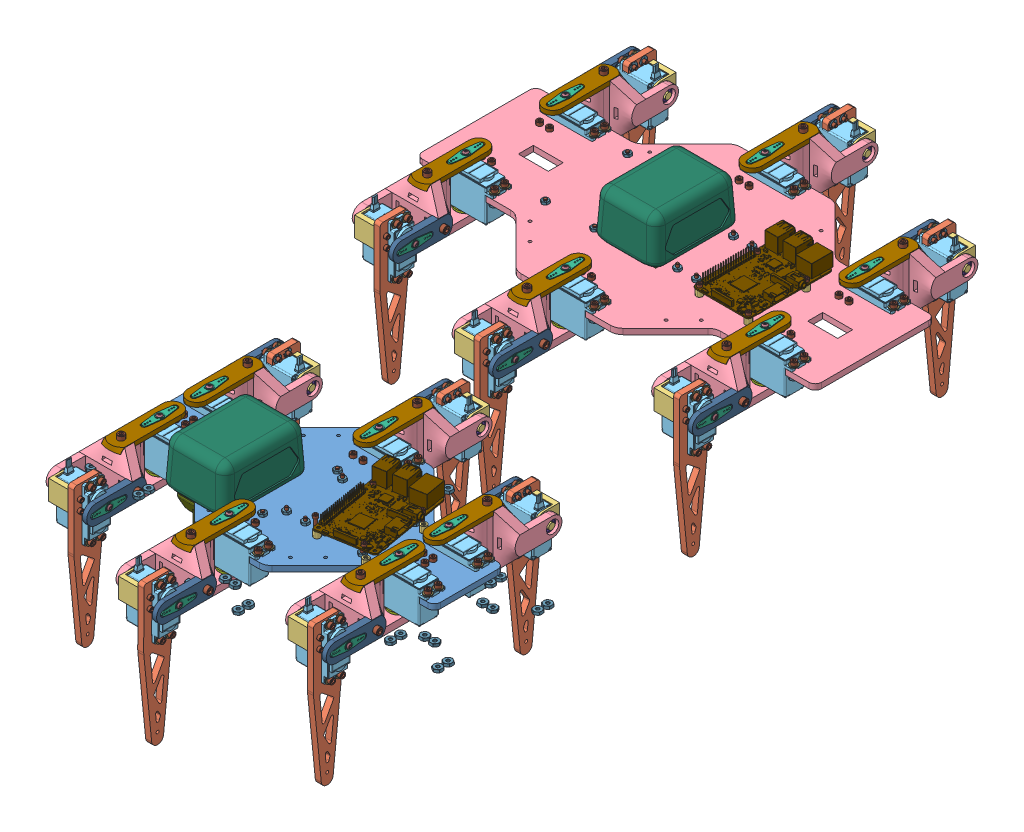
SolidWorks assembly Assem1, configuration Default. Lengths in mm. (continued)
Components (placement in the parent): (continued)
- Hexapod-1: Hexapod [Défaut] at (0 0 -431.8) size (400 181.88 399.28) (continued)
  - Leg_V2(Mirror)-5: Leg_V2(Mirror) [Default] at (-69.94 -26.67 80.094) x (-1 0 0) z (0 0 -1) size (66.23 158.62 124.7) (continued)
    - Joint_attachment_foot-1: Joint_attachment_foot [Défaut] at (17.1065 26.4662 -54.3509) x (0.000191 0 -1) z (0 1 0) size (64.08 6.7 19.07)
    - socket_1_2_6-32_with_washer-1: socket_1_2_6-32_with_washer [Défaut] at (25.0085 -14.6702 -93.4398) x (1 0 0.000191) z (-0.000165 -0.501262 0.865296) size (16.21 7.92 7.92)
      - socket head cap screw_ai-1: socket head cap screw_ai [HX-SHCS 0.138-32x0.5x0.5-N] at (-51.206 -1.62 2.0257) size (16.21 5.74 5.74)
      - flat washer type b narrow_ai-1: flat washer type b narrow_ai [Narrow FW 0.138] at (-46.888 -1.62 2.0257) size (0.81 7.92 7.92)
    - socket_1_2_6-32_with_washer-2: socket_1_2_6-32_with_washer [Défaut] at (25.0067 -19.1255 -83.9619) x (1 0 0.000191) z (0 0.999999 0.001458) size (16.21 7.92 7.92)
      - socket head cap screw_ai-1: socket head cap screw_ai [HX-SHCS 0.138-32x0.5x0.5-N] at (-51.206 -1.62 2.0257) size (16.21 5.74 5.74)
      - flat washer type b narrow_ai-1: flat washer type b narrow_ai [Narrow FW 0.138] at (-46.888 -1.62 2.0257) size (0.81 7.92 7.92)
    - socket_1_2_6-32_with_washer-3: socket_1_2_6-32_with_washer [Défaut] at (25.0081 27.9935 -91.489) x (1 0 0.000191) z (0.000165 0.501262 -0.865296) size (16.21 7.92 7.92)
      - socket head cap screw_ai-1: socket head cap screw_ai [HX-SHCS 0.138-32x0.5x0.5-N] at (-51.206 -1.62 2.0257) size (16.21 5.74 5.74)
      - flat washer type b narrow_ai-1: flat washer type b narrow_ai [Narrow FW 0.138] at (-46.888 -1.62 2.0257) size (0.81 7.92 7.92)
    - socket_1_2_6-32_with_washer-4: socket_1_2_6-32_with_washer [Défaut] at (25.0062 27.9806 -81.329) x (1 0 0.000191) z (0.000165 0.501262 -0.865296) size (16.21 7.92 7.92)
      - socket head cap screw_ai-1: socket head cap screw_ai [HX-SHCS 0.138-32x0.5x0.5-N] at (-51.206 -1.62 2.0257) size (16.21 5.74 5.74)
      - flat washer type b narrow_ai-1: flat washer type b narrow_ai [Narrow FW 0.138] at (-46.888 -1.62 2.0257) size (0.81 7.92 7.92)
    - socket button head cap screw_ai-2: socket button head cap screw_ai [SBHCSCREW 0.112-40x0.25-HX-N] at (-38.2675 16.9412 -87.3815) x (1 0 0.000191) z (0.000095 0.866025 -0.5) size (7.85 5.41 5.41)
    - socket button head cap screw_ai-3: socket button head cap screw_ai [SBHCSCREW 0.112-40x0.25-HX-N] at (-9.652 45.5715 -9.906) x (0 -1 0) z (0.86593 0 0.500165) size (7.85 5.41 5.41)
    - machine screw nut hex_ai-7: machine screw nut hex_ai [MSHXNUT 0.138-32-D-N] at (-13.365 -17.0874 -92.5063) x (0.000165 0.501262 -0.865296) z (1 0 0.000191) size (7.92 9.15 2.9)
    - machine screw nut hex_ai-8: machine screw nut hex_ai [MSHXNUT 0.138-32-D-N] at (-13.367 -17.1022 -82.3463) x (0.000165 0.501262 -0.865296) z (-1 0 -0.000191) size (7.92 9.15 2.9)
    - machine screw nut hex_ai-9: machine screw nut hex_ai [MSHXNUT 0.138-32-D-N] at (-13.3651 30.4106 -92.4371) x (0 0.999999 0.001458) z (1 0 0.000191) size (7.92 9.15 2.9)
    - machine screw nut hex_ai-10: machine screw nut hex_ai [MSHXNUT 0.138-32-D-N] at (-13.367 30.3978 -82.2771) x (0 0.999999 0.001458) z (1 0 0.000191) size (7.92 9.15 2.9)
    - socket head cap screw_ai-1: socket head cap screw_ai [HX-SHCS 0.164-32x0.5x0.5-N] at (-9.6447 47.8568 -48.4039) x (0 -1 0) z (-0.000191 0 1) size (16.87 6.86 6.86)
    - socket head cap screw_ai-2: socket head cap screw_ai [HX-SHCS 0.164-32x0.5x0.5-N] at (-40.5581 16.9412 -59.655) x (1 0 0.000191) z (-0.000191 0 1) size (16.87 6.86 6.86)
    - machine screw nut hex_ai-11: machine screw nut hex_ai [MSHXNUT 0.164-32-D-N] at (-9.6447 33.127 -48.4039) x (0.86593 0 0.500165) z (0 1 0) size (8.74 10.09 3.3)
    - machine screw nut hex_ai-12: machine screw nut hex_ai [MSHXNUT 0.164-32-D-N] at (-25.8283 16.9412 -59.6522) x (-0.000191 0 1) z (-1 0 -0.000191) size (8.74 10.09 3.3)
    - socket head cap screw_ai-3: socket head cap screw_ai [HX-SHCS 0.112-40x0.5x0.5-N] at (-22.2084 11.6733 -99.7961) x (1 0 0.000191) z (-0.000191 -0.001458 0.999999) size (15.54 4.65 4.65)
    - socket head cap screw_ai-4: socket head cap screw_ai [HX-SHCS 0.112-40x0.5x0.5-N] at (-22.2084 21.6733 -99.7815) x (1 0 0.000191) z (0.000191 0.001458 -0.999999) size (15.54 4.65 4.65)
    - socket_1_2_6-32_with_washer-5: socket_1_2_6-32_with_washer [Défaut] at (3.4199 -17.7034 -12.4217) x (0 -1 0) z (-0.5 0 -0.866025) size (16.21 7.92 7.92)
      - socket head cap screw_ai-1: socket head cap screw_ai [HX-SHCS 0.138-32x0.5x0.5-N] at (-51.206 -1.62 2.0257) size (16.21 5.74 5.74)
      - flat washer type b narrow_ai-1: flat washer type b narrow_ai [Narrow FW 0.138] at (-46.888 -1.62 2.0257) size (0.81 7.92 7.92)
    - socket_1_2_6-32_with_washer-6: socket_1_2_6-32_with_washer [Défaut] at (-44.0781 -17.7034 -2.2617) x (0 -1 0) z (-0.5 0 -0.866025) size (16.21 7.92 7.92)
      - socket head cap screw_ai-1: socket head cap screw_ai [HX-SHCS 0.138-32x0.5x0.5-N] at (-51.206 -1.62 2.0257) size (16.21 5.74 5.74)
      - flat washer type b narrow_ai-1: flat washer type b narrow_ai [Narrow FW 0.138] at (-46.888 -1.62 2.0257) size (0.81 7.92 7.92)
    - socket_1_2_6-32_with_washer-7: socket_1_2_6-32_with_washer [Défaut] at (3.4199 -17.7034 -2.2617) x (0 -1 0) z (-0.5 0 -0.866025) size (16.21 7.92 7.92)
      - socket head cap screw_ai-1: socket head cap screw_ai [HX-SHCS 0.138-32x0.5x0.5-N] at (-51.206 -1.62 2.0257) size (16.21 5.74 5.74)
      - flat washer type b narrow_ai-1: flat washer type b narrow_ai [Narrow FW 0.138] at (-46.888 -1.62 2.0257) size (0.81 7.92 7.92)
    - socket_1_2_6-32_with_washer-8: socket_1_2_6-32_with_washer [Défaut] at (-44.0781 -17.7034 -12.4217) x (0 -1 0) z (-0.5 0 -0.866025) size (16.21 7.92 7.92)
      - socket head cap screw_ai-1: socket head cap screw_ai [HX-SHCS 0.138-32x0.5x0.5-N] at (-51.206 -1.62 2.0257) size (16.21 5.74 5.74)
      - flat washer type b narrow_ai-1: flat washer type b narrow_ai [Narrow FW 0.138] at (-46.888 -1.62 2.0257) size (0.81 7.92 7.92)
  - Leg_V2(Mirror)-6: Leg_V2(Mirror) [Default] at (-219.94 -26.67 130.094) x (-1 0 0) z (0 0 -1) size (66.23 158.62 124.7)
    - Foot_V2_Straight-1: Foot_V2_Straight [Default] at (-13.3652 4.661 -91.3946) x (-0.000191 -0.001458 0.999999) z (-1 0 -0.000191) size (28 145.4 6)
    - bearing_mount_foot-1: bearing_mount_foot [Default] at (-13.1936 16.6093 -99.7872) x (0.000191 0.001458 -0.999999) z (1 0 0.000191) size (25 20 29.5)
    - Joint-1: Joint [Défaut] at (17.1065 26.4662 -54.3509) x (0.000191 0 -1) z (0 1 0) size (96.52 53.26 53.26)
    - hs-422-2: hs-422 [Défaut] at (-13.3989 6.6398 -77.4857) x (0.000191 0.001458 -0.999999) z (0 0.999999 0.001458) size (19.81 42.09 58.23)
    - hs-422-3: hs-422 [Défaut] at (-19.939 20.701 0) x (0 0 -1) z (1 0 0) size (19.81 42.09 58.23)
    - hs-422_horn_straight-1: hs-422_horn_straight [Default] at (-35.2703 16.9412 -87.3809) x (-0.000191 0 1) z (0 1 0) size (33.93 4.93 8.79)
    - hs-422_horn_straight-2: hs-422_horn_straight [Default] at (-9.652 42.5743 -9.906) x (0.000191 0 -1) z (-1 0 -0.000191) size (33.93 4.93 8.79)
    - Bearing_mount_leg-1: Bearing_mount_leg [Default] at (-9.652 21 2.594) x (0 0 1) z (0 -1 0) size (35 20 30)
    - Bearing-1: Bearing [Default] at (-9.652 -6.7498 -9.906) x (0.84763 0 0.530588) z (-0.530588 0 0.84763) size (13.87 4.75 13.87)
    - Bearing-2: Bearing [Default] at (14.0538 16.9412 -87.3715) x (-0.000107 0.826531 0.562891) z (-0.000158 -0.562891 0.826531) size (13.87 4.75 13.87)
    - Joint_attachment_leg-1: Joint_attachment_leg [Défaut] at (17.1065 26.4662 -54.3509) x (0.000191 0 -1) z (0 1 0) size (74.32 19.07 4.32)
    - Joint_attachment_foot-1: Joint_attachment_foot [Défaut] at (17.1065 26.4662 -54.3509) x (0.000191 0 -1) z (0 1 0) size (64.08 6.7 19.07)
    - socket_1_2_6-32_with_washer-1: socket_1_2_6-32_with_washer [Défaut] at (25.0085 -14.6702 -93.4398) x (1 0 0.000191) z (-0.000165 -0.501262 0.865296) size (16.21 7.92 7.92)
      - socket head cap screw_ai-1: socket head cap screw_ai [HX-SHCS 0.138-32x0.5x0.5-N] at (-51.206 -1.62 2.0257) size (16.21 5.74 5.74)
      - flat washer type b narrow_ai-1: flat washer type b narrow_ai [Narrow FW 0.138] at (-46.888 -1.62 2.0257) size (0.81 7.92 7.92)
    - socket_1_2_6-32_with_washer-2: socket_1_2_6-32_with_washer [Défaut] at (25.0067 -19.1255 -83.9619) x (1 0 0.000191) z (0 0.999999 0.001458) size (16.21 7.92 7.92)
      - socket head cap screw_ai-1: socket head cap screw_ai [HX-SHCS 0.138-32x0.5x0.5-N] at (-51.206 -1.62 2.0257) size (16.21 5.74 5.74)
      - flat washer type b narrow_ai-1: flat washer type b narrow_ai [Narrow FW 0.138] at (-46.888 -1.62 2.0257) size (0.81 7.92 7.92)
    - socket_1_2_6-32_with_washer-3: socket_1_2_6-32_with_washer [Défaut] at (25.0081 27.9935 -91.489) x (1 0 0.000191) z (0.000165 0.501262 -0.865296) size (16.21 7.92 7.92)
      - socket head cap screw_ai-1: socket head cap screw_ai [HX-SHCS 0.138-32x0.5x0.5-N] at (-51.206 -1.62 2.0257) size (16.21 5.74 5.74)
      - flat washer type b narrow_ai-1: flat washer type b narrow_ai [Narrow FW 0.138] at (-46.888 -1.62 2.0257) size (0.81 7.92 7.92)
    - socket_1_2_6-32_with_washer-4: socket_1_2_6-32_with_washer [Défaut] at (25.0062 27.9806 -81.329) x (1 0 0.000191) z (0.000165 0.501262 -0.865296) size (16.21 7.92 7.92)
      - socket head cap screw_ai-1: socket head cap screw_ai [HX-SHCS 0.138-32x0.5x0.5-N] at (-51.206 -1.62 2.0257) size (16.21 5.74 5.74)
      - flat washer type b narrow_ai-1: flat washer type b narrow_ai [Narrow FW 0.138] at (-46.888 -1.62 2.0257) size (0.81 7.92 7.92)
    - socket button head cap screw_ai-2: socket button head cap screw_ai [SBHCSCREW 0.112-40x0.25-HX-N] at (-38.2675 16.9412 -87.3815) x (1 0 0.000191) z (0.000095 0.866025 -0.5) size (7.85 5.41 5.41)
    - socket button head cap screw_ai-3: socket button head cap screw_ai [SBHCSCREW 0.112-40x0.25-HX-N] at (-9.652 45.5715 -9.906) x (0 -1 0) z (0.86593 0 0.500165) size (7.85 5.41 5.41)
    - machine screw nut hex_ai-7: machine screw nut hex_ai [MSHXNUT 0.138-32-D-N] at (-13.365 -17.0874 -92.5063) x (0.000165 0.501262 -0.865296) z (1 0 0.000191) size (7.92 9.15 2.9)
    - machine screw nut hex_ai-8: machine screw nut hex_ai [MSHXNUT 0.138-32-D-N] at (-13.367 -17.1022 -82.3463) x (0.000165 0.501262 -0.865296) z (-1 0 -0.000191) size (7.92 9.15 2.9)
    - machine screw nut hex_ai-9: machine screw nut hex_ai [MSHXNUT 0.138-32-D-N] at (-13.3651 30.4106 -92.4371) x (0 0.999999 0.001458) z (1 0 0.000191) size (7.92 9.15 2.9)
    - machine screw nut hex_ai-10: machine screw nut hex_ai [MSHXNUT 0.138-32-D-N] at (-13.367 30.3978 -82.2771) x (0 0.999999 0.001458) z (1 0 0.000191) size (7.92 9.15 2.9)
    - socket head cap screw_ai-1: socket head cap screw_ai [HX-SHCS 0.164-32x0.5x0.5-N] at (-9.6447 47.8568 -48.4039) x (0 -1 0) z (-0.000191 0 1) size (16.87 6.86 6.86)
    - socket head cap screw_ai-2: socket head cap screw_ai [HX-SHCS 0.164-32x0.5x0.5-N] at (-40.5581 16.9412 -59.655) x (1 0 0.000191) z (-0.000191 0 1) size (16.87 6.86 6.86)
    - machine screw nut hex_ai-11: machine screw nut hex_ai [MSHXNUT 0.164-32-D-N] at (-9.6447 33.127 -48.4039) x (0.86593 0 0.500165) z (0 1 0) size (8.74 10.09 3.3)
    - machine screw nut hex_ai-12: machine screw nut hex_ai [MSHXNUT 0.164-32-D-N] at (-25.8283 16.9412 -59.6522) x (-0.000191 0 1) z (-1 0 -0.000191) size (8.74 10.09 3.3)
    - socket head cap screw_ai-3: socket head cap screw_ai [HX-SHCS 0.112-40x0.5x0.5-N] at (-22.2084 11.6733 -99.7961) x (1 0 0.000191) z (-0.000191 -0.001458 0.999999) size (15.54 4.65 4.65)
    - socket head cap screw_ai-4: socket head cap screw_ai [HX-SHCS 0.112-40x0.5x0.5-N] at (-22.2084 21.6733 -99.7815) x (1 0 0.000191) z (0.000191 0.001458 -0.999999) size (15.54 4.65 4.65)
    - socket_1_2_6-32_with_washer-5: socket_1_2_6-32_with_washer [Défaut] at (3.4199 -17.7034 -12.4217) x (0 -1 0) z (-0.5 0 -0.866025) size (16.21 7.92 7.92)
      - socket head cap screw_ai-1: socket head cap screw_ai [HX-SHCS 0.138-32x0.5x0.5-N] at (-51.206 -1.62 2.0257) size (16.21 5.74 5.74)
      - flat washer type b narrow_ai-1: flat washer type b narrow_ai [Narrow FW 0.138] at (-46.888 -1.62 2.0257) size (0.81 7.92 7.92)
    - socket_1_2_6-32_with_washer-6: socket_1_2_6-32_with_washer [Défaut] at (-44.0781 -17.7034 -2.2617) x (0 -1 0) z (-0.5 0 -0.866025) size (16.21 7.92 7.92)
      - socket head cap screw_ai-1: socket head cap screw_ai [HX-SHCS 0.138-32x0.5x0.5-N] at (-51.206 -1.62 2.0257) size (16.21 5.74 5.74)
      - flat washer type b narrow_ai-1: flat washer type b narrow_ai [Narrow FW 0.138] at (-46.888 -1.62 2.0257) size (0.81 7.92 7.92)
    - socket_1_2_6-32_with_washer-7: socket_1_2_6-32_with_washer [Défaut] at (3.4199 -17.7034 -2.2617) x (0 -1 0) z (-0.5 0 -0.866025) size (16.21 7.92 7.92)
      - socket head cap screw_ai-1: socket head cap screw_ai [HX-SHCS 0.138-32x0.5x0.5-N] at (-51.206 -1.62 2.0257) size (16.21 5.74 5.74)
      - flat washer type b narrow_ai-1: flat washer type b narrow_ai [Narrow FW 0.138] at (-46.888 -1.62 2.0257) size (0.81 7.92 7.92)
    - socket_1_2_6-32_with_washer-8: socket_1_2_6-32_with_washer [Défaut] at (-44.0781 -17.7034 -12.4217) x (0 -1 0) z (-0.5 0 -0.866025) size (16.21 7.92 7.92)
      - socket head cap screw_ai-1: socket head cap screw_ai [HX-SHCS 0.138-32x0.5x0.5-N] at (-51.206 -1.62 2.0257) size (16.21 5.74 5.74)
      - flat washer type b narrow_ai-1: flat washer type b narrow_ai [Narrow FW 0.138] at (-46.888 -1.62 2.0257) size (0.81 7.92 7.92)
  - Battery-1: Battery [Défaut] at (-209.6397 14.6626 -46.247) x (-1 0 0) z (0 0 1) size (64.47 74.3 85.78)
    - MAKITA 4.0AH-1: MAKITA 4.0AH [Défaut] at (0.5853 -29.7874 85.4436) size (64.47 57.15 85.78)
    - MAKITA 4.0AH MOBILE-1: MAKITA 4.0AH MOBILE [Défaut] at (0.5853 -39.3124 91.7936) size (45.84 26.68 66.29)
  - arduinoMega-1: arduinoMega [Detailed] at (-270.251 -7.6 40.62) x (0 0 -1) z (-1 0 0) size (108.32 14.5 53.3)
  - raspberryPi3B-1: raspberryPi3B [Detailed] at (-112.5 6.35 40) x (0 0 -1) z (0 1 0) size (87.05 58.5 19.5)
  - 12Channel PWM-1: 12Channel PWM [Default] at (-160.6 -5.6 40) x (-1 0 0) z (0 0 1) size (25.4 7.55 66.7)
  - DROK_090483.stp-1: DROK_090483.stp [Default] at (-90.995 -5.6 69.895) x (-1 0 0) z (0 -1 0) size (50.02 60 18.9)
  - socket head cap screw_ai-2: socket head cap screw_ai [HX-SHCS 0.138-32x0.625x0.625-N] at (-55.288 3.5052 69.09) x (0 -1 0) z (1 0 0) size (19.38 5.74 5.74)
  - socket head cap screw_ai-3: socket head cap screw_ai [HX-SHCS 0.138-32x0.625x0.625-N] at (-65.288 3.5052 69.09) x (0 -1 0) z (0.5 0 0.866025) size (19.38 5.74 5.74)
  - socket head cap screw_ai-4: socket head cap screw_ai [HX-SHCS 0.138-32x0.625x0.625-N] at (-65.288 3.5052 10.91) x (0 -1 0) z (1 0 0) size (19.38 5.74 5.74)
  - socket head cap screw_ai-5: socket head cap screw_ai [HX-SHCS 0.138-32x0.625x0.625-N] at (-55.288 3.5052 10.91) x (0 -1 0) z (1 0 0) size (19.38 5.74 5.74)
  - socket head cap screw_ai-6: socket head cap screw_ai [HX-SHCS 0.138-32x0.625x0.625-N] at (-215.288 3.5052 119.09) x (0 -1 0) z (1 0 0) size (19.38 5.74 5.74)
  - socket head cap screw_ai-7: socket head cap screw_ai [HX-SHCS 0.138-32x0.625x0.625-N] at (-205.288 3.5052 119.09) x (0 -1 0) z (1 0 0) size (19.38 5.74 5.74)
  - socket head cap screw_ai-14: socket head cap screw_ai [HX-SHCS 0.138-32x0.625x0.625-N] at (-205.288 3.5052 -39.09) x (0 -1 0) z (1 0 0) size (19.38 5.74 5.74)
  - socket head cap screw_ai-15: socket head cap screw_ai [HX-SHCS 0.138-32x0.625x0.625-N] at (-215.288 3.5052 -39.09) x (0 -1 0) z (1 0 0) size (19.38 5.74 5.74)
  - socket head cap screw_ai-16: socket head cap screw_ai [HX-SHCS 0.138-32x0.625x0.625-N] at (-355.288 3.5052 69.09) x (0 -1 0) z (1 0 0) size (19.38 5.74 5.74)
  - socket head cap screw_ai-17: socket head cap screw_ai [HX-SHCS 0.138-32x0.625x0.625-N] at (-365.288 3.5052 69.09) x (0 -1 0) z (0.5 0 0.866025) size (19.38 5.74 5.74)
  - socket head cap screw_ai-18: socket head cap screw_ai [HX-SHCS 0.138-32x0.625x0.625-N] at (-365.288 3.5052 10.91) x (0 -1 0) z (1 0 0) size (19.38 5.74 5.74)
  - socket head cap screw_ai-19: socket head cap screw_ai [HX-SHCS 0.138-32x0.625x0.625-N] at (-355.288 3.5052 10.91) x (0 -1 0) z (1 0 0) size (19.38 5.74 5.74)
  - machine screw nut hex_ai-60: machine screw nut hex_ai [MSHXNUT 0.138-32-D-N] at (-373.75 -8.4956 -15.08) x (1 0 0) z (0 -1 0) size (7.92 9.15 2.9)
  - machine screw nut hex_ai-65: machine screw nut hex_ai [MSHXNUT 0.138-32-D-N] at (-373.75 -8.4956 -4.92) x (1 0 0) z (0 -1 0) size (7.92 9.15 2.9)
  - machine screw nut hex_ai-70: machine screw nut hex_ai [MSHXNUT 0.138-32-D-N] at (-326.252 -8.4956 -4.92) x (0.5 0 0.866025) z (0 -1 0) size (7.92 9.15 2.9)
  - machine screw nut hex_ai-75: machine screw nut hex_ai [MSHXNUT 0.138-32-D-N] at (-326.252 -8.4956 -15.08) x (0.5 0 0.866025) z (0 -1 0) size (7.92 9.15 2.9)
  - machine screw nut hex_ai-80: machine screw nut hex_ai [MSHXNUT 0.138-32-D-N] at (-355.288 -13.5656 10.91) x (0 0 1) z (0 -1 0) size (7.92 9.15 2.9)
  - machine screw nut hex_ai-85: machine screw nut hex_ai [MSHXNUT 0.138-32-D-N] at (-365.288 -13.5656 10.91) x (0 0 1) z (0 -1 0) size (7.92 9.15 2.9)
  - machine screw nut hex_ai-63: machine screw nut hex_ai [MSHXNUT 0.138-32-D-N] at (-223.75 -8.4956 -65.08) x (1 0 0) z (0 -1 0) size (7.92 9.15 2.9)
  - machine screw nut hex_ai-68: machine screw nut hex_ai [MSHXNUT 0.138-32-D-N] at (-223.75 -8.4956 -54.92) x (1 0 0) z (0 -1 0) size (7.92 9.15 2.9)
  - machine screw nut hex_ai-73: machine screw nut hex_ai [MSHXNUT 0.138-32-D-N] at (-176.252 -8.4956 -54.92) x (0.5 0 0.866025) z (0 -1 0) size (7.92 9.15 2.9)
  - machine screw nut hex_ai-78: machine screw nut hex_ai [MSHXNUT 0.138-32-D-N] at (-176.252 -8.4956 -65.08) x (0.5 0 0.866025) z (0 -1 0) size (7.92 9.15 2.9)
  - machine screw nut hex_ai-83: machine screw nut hex_ai [MSHXNUT 0.138-32-D-N] at (-205.288 -13.5656 -39.09) x (0 0 1) z (0 -1 0) size (7.92 9.15 2.9)
  - machine screw nut hex_ai-86: machine screw nut hex_ai [MSHXNUT 0.138-32-D-N] at (-215.288 -13.5656 -39.09) x (0 0 1) z (0 -1 0) size (7.92 9.15 2.9)
  - machine screw nut hex_ai-87: machine screw nut hex_ai [MSHXNUT 0.138-32-D-N] at (-65.288 -13.5656 10.91) x (0 0 1) z (0 -1 0) size (7.92 9.15 2.9)
  - machine screw nut hex_ai-84: machine screw nut hex_ai [MSHXNUT 0.138-32-D-N] at (-55.288 -13.5656 10.91) x (0 0 1) z (0 -1 0) size (7.92 9.15 2.9)
  - machine screw nut hex_ai-74: machine screw nut hex_ai [MSHXNUT 0.138-32-D-N] at (-26.252 -8.4956 -4.92) x (0.5 0 0.866025) z (0 -1 0) size (7.92 9.15 2.9)
  - machine screw nut hex_ai-79: machine screw nut hex_ai [MSHXNUT 0.138-32-D-N] at (-26.252 -8.4956 -15.08) x (0.5 0 0.866025) z (0 -1 0) size (7.92 9.15 2.9)
  - machine screw nut hex_ai-69: machine screw nut hex_ai [MSHXNUT 0.138-32-D-N] at (-73.75 -8.4956 -4.92) x (1 0 0) z (0 -1 0) size (7.92 9.15 2.9)
  - machine screw nut hex_ai-64: machine screw nut hex_ai [MSHXNUT 0.138-32-D-N] at (-73.75 -8.4956 -15.08) x (1 0 0) z (0 -1 0) size (7.92 9.15 2.9)
  - machine screw nut hex_ai-88: machine screw nut hex_ai [MSHXNUT 0.138-32-D-N] at (-365.288 -10.67 69.09) x (0 0 -1) z (0 1 0) size (7.92 9.15 2.9)
  - machine screw nut hex_ai-89: machine screw nut hex_ai [MSHXNUT 0.138-32-D-N] at (-355.288 -10.67 69.09) x (0 0 -1) z (0 1 0) size (7.92 9.15 2.9)
  - machine screw nut hex_ai-90: machine screw nut hex_ai [MSHXNUT 0.138-32-D-N] at (-326.252 -5.6 84.92) x (0.5 0 -0.866025) z (0 1 0) size (7.92 9.15 2.9)
  - machine screw nut hex_ai-91: machine screw nut hex_ai [MSHXNUT 0.138-32-D-N] at (-326.252 -5.6 95.08) x (0.5 0 -0.866025) z (0 1 0) size (7.92 9.15 2.9)
  - machine screw nut hex_ai-92: machine screw nut hex_ai [MSHXNUT 0.138-32-D-N] at (-373.75 -5.6 84.92) x (1 0 0) z (0 1 0) size (7.92 9.15 2.9)
  - machine screw nut hex_ai-93: machine screw nut hex_ai [MSHXNUT 0.138-32-D-N] at (-373.75 -5.6 95.08) x (1 0 0) z (0 1 0) size (7.92 9.15 2.9)
  - machine screw nut hex_ai-94: machine screw nut hex_ai [MSHXNUT 0.138-32-D-N] at (-223.75 -5.6 145.08) x (1 0 0) z (0 1 0) size (7.92 9.15 2.9)
  - machine screw nut hex_ai-95: machine screw nut hex_ai [MSHXNUT 0.138-32-D-N] at (-223.75 -5.6 134.92) x (1 0 0) z (0 1 0) size (7.92 9.15 2.9)
  - machine screw nut hex_ai-96: machine screw nut hex_ai [MSHXNUT 0.138-32-D-N] at (-176.252 -5.6 134.92) x (0.5 0 -0.866025) z (0 1 0) size (7.92 9.15 2.9)
  - machine screw nut hex_ai-97: machine screw nut hex_ai [MSHXNUT 0.138-32-D-N] at (-176.252 -5.6 145.08) x (0.5 0 -0.866025) z (0 1 0) size (7.92 9.15 2.9)
  - machine screw nut hex_ai-98: machine screw nut hex_ai [MSHXNUT 0.138-32-D-N] at (-205.288 -10.67 119.09) x (0 0 -1) z (0 1 0) size (7.92 9.15 2.9)
  - machine screw nut hex_ai-99: machine screw nut hex_ai [MSHXNUT 0.138-32-D-N] at (-215.288 -10.67 119.09) x (0 0 -1) z (0 1 0) size (7.92 9.15 2.9)
  - machine screw nut hex_ai-100: machine screw nut hex_ai [MSHXNUT 0.138-32-D-N] at (-65.288 -10.67 69.09) x (0 0 -1) z (0 1 0) size (7.92 9.15 2.9)
  - machine screw nut hex_ai-101: machine screw nut hex_ai [MSHXNUT 0.138-32-D-N] at (-55.288 -10.67 69.09) x (0 0 -1) z (0 1 0) size (7.92 9.15 2.9)
  - machine screw nut hex_ai-102: machine screw nut hex_ai [MSHXNUT 0.138-32-D-N] at (-26.252 -5.6 84.92) x (0.5 0 -0.866025) z (0 1 0) size (7.92 9.15 2.9)
  - machine screw nut hex_ai-103: machine screw nut hex_ai [MSHXNUT 0.138-32-D-N] at (-26.252 -5.6 95.08) x (0.5 0 -0.866025) z (0 1 0) size (7.92 9.15 2.9)
  - machine screw nut hex_ai-104: machine screw nut hex_ai [MSHXNUT 0.138-32-D-N] at (-73.75 -5.6 84.92) x (1 0 0) z (0 1 0) size (7.92 9.15 2.9)
  - machine screw nut hex_ai-105: machine screw nut hex_ai [MSHXNUT 0.138-32-D-N] at (-73.75 -5.6 95.08) x (1 0 0) z (0 1 0) size (7.92 9.15 2.9)
  - socket head cap screw_ai-20: socket head cap screw_ai [HX-SHCS 0.138-32x0.5x0.5-N] at (-246.141 -12.6052 74.88) x (0 1 0) z (-0.5 0 -0.866025) size (16.21 5.74 5.74)
  - socket head cap screw_ai-21: socket head cap screw_ai [HX-SHCS 0.138-32x0.5x0.5-N] at (-294.361 -12.6052 -6.36) x (0 1 0) z (1 0 0) size (16.21 5.74 5.74)
  - socket head cap screw_ai-22: socket head cap screw_ai [HX-SHCS 0.138-32x0.5x0.5-N] at (-246.141 -12.6052 0) x (0 1 0) z (-0.5 0 -0.866025) size (16.21 5.74 5.74)
  - socket head cap screw_ai-23: socket head cap screw_ai [HX-SHCS 0.138-32x0.5x0.5-N] at (-294.361 -12.6052 76.11) x (0 1 0) z (-1 0 0) size (16.21 5.74 5.74)
  - machine screw nut hex_ai-106: machine screw nut hex_ai [MSHXNUT 0.112-40-D-N] at (-294.361 2.4892 -6.36) x (1 0 0) z (0 1 0) size (6.35 7.33 2.49)
  - machine screw nut hex_ai-107: machine screw nut hex_ai [MSHXNUT 0.112-40-D-N] at (-294.361 2.4892 76.11) x (1 0 0) z (0 1 0) size (6.35 7.33 2.49)
  - machine screw nut hex_ai-108: machine screw nut hex_ai [MSHXNUT 0.112-40-D-N] at (-246.141 2.4892 0) x (1 0 0) z (0 1 0) size (6.35 7.33 2.49)
  - machine screw nut hex_ai-109: machine screw nut hex_ai [MSHXNUT 0.112-40-D-N] at (-246.141 2.4892 74.88) x (1 0 0) z (0 1 0) size (6.35 7.33 2.49)
  - socket head cap screw_ai-24: socket head cap screw_ai [HX-SHCS 0.138-32x0.5x0.5-N] at (-130.81 -10.3052 13.48) x (0 1 0) z (-0.5 0 -0.866025) size (16.21 5.74 5.74)
  - machine screw nut hex_ai-110: machine screw nut hex_ai [MSHXNUT 0.112-40-D-N] at (-130.81 2.4892 13.48) x (1 0 0) z (0 1 0) size (6.35 7.33 2.49)
  - socket head cap screw_ai-25: socket head cap screw_ai [HX-SHCS 0.138-32x0.5x0.5-N] at (-94.18 -10.3052 13.48) x (0 1 0) z (-0.5 0 -0.866025) size (16.21 5.74 5.74)
  - socket head cap screw_ai-26: socket head cap screw_ai [HX-SHCS 0.138-32x0.5x0.5-N] at (-130.81 -10.3052 66.31) x (0 1 0) z (-0.5 0 -0.866025) size (16.21 5.74 5.74)
  - socket head cap screw_ai-27: socket head cap screw_ai [HX-SHCS 0.138-32x0.5x0.5-N] at (-94.18 -10.3052 66.31) x (0 1 0) z (-0.5 0 -0.866025) size (16.21 5.74 5.74)
  - machine screw nut hex_ai-111: machine screw nut hex_ai [MSHXNUT 0.112-40-D-N] at (-94.18 2.4892 13.48) x (1 0 0) z (0 1 0) size (6.35 7.33 2.49)
  - machine screw nut hex_ai-112: machine screw nut hex_ai [MSHXNUT 0.112-40-D-N] at (-130.81 2.4892 66.31) x (1 0 0) z (0 1 0) size (6.35 7.33 2.49)
  - machine screw nut hex_ai-113: machine screw nut hex_ai [MSHXNUT 0.112-40-D-N] at (-94.18 2.4892 66.31) x (1 0 0) z (0 1 0) size (6.35 7.33 2.49)
  - 1_4_Round_Aluminum_Standoff.step-1: 1_4_Round_Aluminum_Standoff.step [Défaut] at (-88 0 21) x (0.963282 0 -0.268492) z (0.268492 0 0.963282) size (6.34 6.36 6.34)
  - socket head cap screw_ai-28: socket head cap screw_ai [HX-SHCS 0.112-40x1x0.75-N] at (-88 10.4948 21) x (0 -1 0) z (0.5 0 0.866025) size (28.24 4.65 4.65)
  - machine screw nut hex_ai-114: machine screw nut hex_ai [MSHXNUT 0.112-40-D-N] at (-88 -8.0892 21) x (1 0 0) z (0 -1 0) size (6.35 7.33 2.49)
  - 1_4_Round_Aluminum_Standoff.step-2: 1_4_Round_Aluminum_Standoff.step [Défaut] at (-137 0 21) x (0.963282 0 -0.268492) z (0.268492 0 0.963282) size (6.34 6.36 6.34)
  - 1_4_Round_Aluminum_Standoff.step-3: 1_4_Round_Aluminum_Standoff.step [Défaut] at (-88 0 79) x (0.963282 0 -0.268492) z (0.268492 0 0.963282) size (6.34 6.36 6.34)
  - 1_4_Round_Aluminum_Standoff.step-4: 1_4_Round_Aluminum_Standoff.step [Défaut] at (-137 0 79) x (0.963282 0 -0.268492) z (0.268492 0 0.963282) size (6.34 6.36 6.34)
  - machine screw nut hex_ai-115: machine screw nut hex_ai [MSHXNUT 0.112-40-D-N] at (-137 -8.0892 21) x (1 0 0) z (0 -1 0) size (6.35 7.33 2.49)
  - machine screw nut hex_ai-116: machine screw nut hex_ai [MSHXNUT 0.112-40-D-N] at (-88 -8.0892 79) x (1 0 0) z (0 -1 0) size (6.35 7.33 2.49)
  - machine screw nut hex_ai-117: machine screw nut hex_ai [MSHXNUT 0.112-40-D-N] at (-137 -8.0892 79) x (1 0 0) z (0 -1 0) size (6.35 7.33 2.49)
  - socket head cap screw_ai-29: socket head cap screw_ai [HX-SHCS 0.112-40x1x0.75-N] at (-137 10.4948 21) x (0 -1 0) z (0.5 0 0.866025) size (28.24 4.65 4.65)
  - socket head cap screw_ai-30: socket head cap screw_ai [HX-SHCS 0.112-40x1x0.75-N] at (-88 10.4948 79) x (0 -1 0) z (0.5 0 0.866025) size (28.24 4.65 4.65)
  - socket head cap screw_ai-31: socket head cap screw_ai [HX-SHCS 0.112-40x1x0.75-N] at (-137 10.4948 79) x (0 -1 0) z (0.5 0 0.866025) size (28.24 4.65 4.65)
  - socket head cap screw_ai-32: socket head cap screw_ai [HX-SHCS 0.112-40x0.5x0.5-N] at (-170 -9.9448 12.05) x (0 1 0) z (-1 0 0) size (15.54 4.65 4.65)
  - machine screw nut hex_ai-118: machine screw nut hex_ai [MSHXNUT 0.112-40-D-N] at (-170 2.4892 12.05) x (1 0 0) z (0 1 0) size (6.35 7.33 2.49)
  - socket head cap screw_ai-33: socket head cap screw_ai [HX-SHCS 0.112-40x0.5x0.5-N] at (-151.2 -9.9448 12.05) x (0 1 0) z (-1 0 0) size (15.54 4.65 4.65)
  - socket head cap screw_ai-34: socket head cap screw_ai [HX-SHCS 0.112-40x0.5x0.5-N] at (-170 -9.9448 67.95) x (0 1 0) z (-1 0 0) size (15.54 4.65 4.65)
  - socket head cap screw_ai-35: socket head cap screw_ai [HX-SHCS 0.112-40x0.5x0.5-N] at (-151.2 -9.9448 67.95) x (0 1 0) z (-1 0 0) size (15.54 4.65 4.65)
  - machine screw nut hex_ai-119: machine screw nut hex_ai [MSHXNUT 0.112-40-D-N] at (-151.2 2.4892 12.05) x (1 0 0) z (0 1 0) size (6.35 7.33 2.49)
  - machine screw nut hex_ai-120: machine screw nut hex_ai [MSHXNUT 0.112-40-D-N] at (-170 2.4892 67.95) x (1 0 0) z (0 1 0) size (6.35 7.33 2.49)
  - machine screw nut hex_ai-121: machine screw nut hex_ai [MSHXNUT 0.112-40-D-N] at (-151.2 2.4892 67.95) x (1 0 0) z (0 1 0) size (6.35 7.33 2.49)
Mates (geometry in assembly coordinates):
- Coincident3: coincident aligned: plane of Hexapod_NewBody-1 through (0 0 0) normal (0 0 1)
- Coincident4: coincident aligned: plane of Hexapod_NewBody-1 through (0 0 0) normal (0 1 0)
- Coincident5: coincident aligned: plane of Hexapod_NewBody-1 through (0 0 0) normal (1 0 0)
- Distance1: distance = 431.8 mm aligned: plane of Hexapod-1 through (0 0 -431.8) normal (0 0 1)
- Coincident7: coincident aligned: plane of Hexapod-1 through (0 0 -431.8) normal (0 1 0)
- Coincident8: coincident aligned: plane of Hexapod-1 through (0 0 -431.8) normal (1 0 0)
